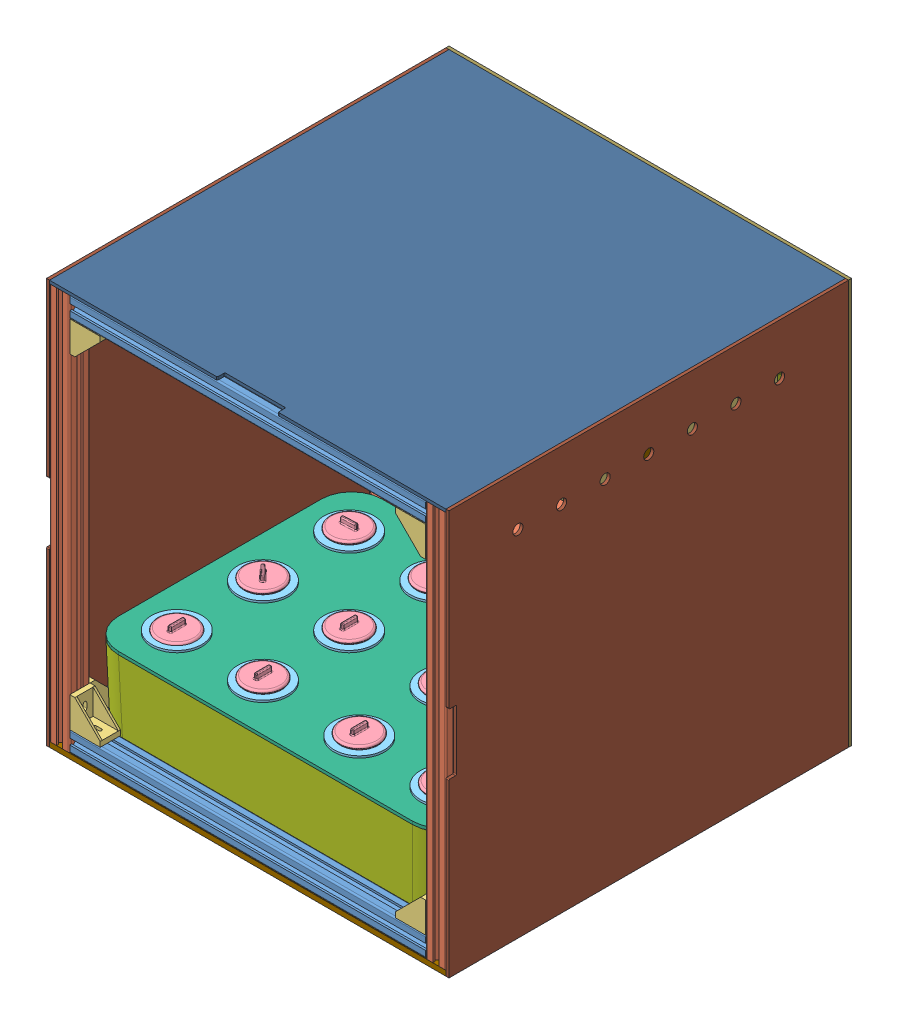
SolidWorks assembly skeleton_v2, configuration 預設. Lengths in mm.
Overall size (397 399 397).
120 component instances, 60 part files, 439 mates.
Components (placement in the parent):
- stick_2020_340-1: stick_2020_340 [預設] at (-3.9446 -1.8678 340) size (20 20 351)
- stick_2020_380-1: stick_2020_380 [預設] at (-3.9446 379.1322 701) x (0 0 1) z (0 -1 0) size (20 20 391)
- stick_2020_340-2: stick_2020_340 [預設] at (357.0554 -1.8678 701) x (0 0 1) z (-1 0 0) size (20 20 351)
- stick_2020_340-3: stick_2020_340 [預設] at (-3.9446 369.1322 340) size (20 20 351)
- stick_2020_340-4: stick_2020_340 [預設] at (357.0554 369.1322 701) x (0 0 1) z (-1 0 0) size (20 20 351)
- stick_2020_340-5: stick_2020_340 [預設] at (357.0554 369.1322 330) x (0 0 1) z (-1 0 0) size (20 20 351)
- stick_2020_340-6: stick_2020_340 [預設] at (367.0554 -1.8678 691) x (-1 0 0) z (0 0 -1) size (20 20 351)
- stick_2020_340-7: stick_2020_340 [預設] at (367.0554 369.1322 691) x (-1 0 0) z (0 0 -1) size (20 20 351)
- stick_2020_340-8: stick_2020_340 [預設] at (6.0554 -1.8678 330) x (0 -1 0) z (1 0 0) size (20 20 351)
- stick_2020_380-2: stick_2020_380 [預設] at (-3.9446 379.1322 330) x (0 0 1) z (0 -1 0) size (20 20 391)
- stick_2020_380-3: stick_2020_380 [預設] at (367.0554 379.1322 701) x (0 0 1) z (0 -1 0) size (20 20 391)
- stick_2020_380-4: stick_2020_380 [預設] at (367.0554 379.1322 330) x (0 0 1) z (0 -1 0) size (20 20 391)
- 零件2^skeleton_v2-1: 零件2^skeleton_v2 [預設] at origin (virtual)
- FixedcomponentWithtriright-2: FixedcomponentWithtriright [預設] at (287.8736 343.8981 342.3593) x (0 -1 0) z (0 0 1) size (81.36 80.18 24)
- small lid-1: small lid [預設] at (48.5554 83.1322 562.9859) x (-0.71803 0 0.696012) z (-0.696012 0 -0.71803) size (38 19 38)
- small lid-2: small lid [預設] at (48.5554 81.1322 647.9859) size (38 19 38)
- small lid-4: small lid [預設] at (228.5554 83.1322 477.9859) x (0.923727 0 0.383052) z (-0.383052 0 0.923727) size (38 19 38)
- small lid-5: small lid [預設] at (228.5554 83.1322 647.9859) size (38 19 38)
- small lid-6: small lid [預設] at (48.5554 83.1322 477.9859) x (0.040502 0 0.999179) z (-0.999179 0 0.040502) size (38 19 38)
- small lid-7: small lid [預設] at (133.5554 83.1322 562.9859) size (38 19 38)
- small lid-8: small lid [預設] at (228.5554 83.1322 562.9859) x (0.921959 0 0.387288) z (-0.387288 0 0.921959) size (38 19 38)
- small lid-9: small lid [預設] at (313.5554 83.1322 647.9859) size (38 19 38)
- small lid-10: small lid [預設] at (133.5554 83.1322 477.9859) x (0.981055 0 -0.193727) z (0.193727 0 0.981055) size (38 19 38)
- small lid-11: small lid [預設] at (133.5554 83.1322 647.9859) size (38 19 38)
- ring-2: ring [預設] at (48.5554 81.1322 562.9859) x (-0.846172 0 0.53291) z (-0.53291 0 -0.846172) size (49.5 5.25 49.5)
- ring-3: ring [預設] at (48.5554 81.1322 647.9859) x (0.619769 0 0.784784) z (-0.784784 0 0.619769) size (49.5 5.25 49.5)
- ring-6: ring [預設] at (133.5554 81.1322 477.9859) x (0.017137 0 0.999853) z (-0.999853 0 0.017137) size (49.5 5.25 49.5)
- ring-9: ring [預設] at (133.5554 81.1322 562.9859) size (49.5 5.25 49.5)
- ring-10: ring [預設] at (133.5554 81.1322 647.9859) x (0.510723 0 0.859745) z (-0.859745 0 0.510723) size (49.5 5.25 49.5)
- ring-11: ring [預設] at (313.5554 81.1322 477.9859) size (49.5 5.25 49.5)
- ring-12: ring [預設] at (313.5554 81.1322 562.9859) size (49.5 5.25 49.5)
- ring-13: ring [預設] at (228.5554 81.1322 647.9859) size (49.5 5.25 49.5)
- ring-14: ring [預設] at (228.5554 81.1322 562.9859) size (49.5 5.25 49.5)
- ring-15: ring [預設] at (228.5554 81.1322 477.9859) size (49.5 5.25 49.5)
- ring-16: ring [預設] at (313.5554 81.1322 647.9859) size (49.5 5.25 49.5)
- ring-17: ring [預設] at (48.5554 81.1322 477.9859) x (0.560642 0 0.828058) z (-0.828058 0 0.560642) size (49.5 5.25 49.5)
- lid_v2-1: lid_v2 [預設] at (181.0554 78.1322 562.9859) size (350 3 260)
- water_tank_v3-1: water_tank_v3 [預設] at (181.0554 -11.8678 562.9859) size (350 90 260)
- small fixed lid with EC sensor and temperture-3: small fixed lid with EC sensor and temperture [預設] at (313.5554 85.1322 562.9859) x (0.682945 0 -0.73047) z (0.73047 0 0.682945) size (38.59 9 40.38)
- plate_bottom-1: plate_bottom [預設] at (181.5554 -16.8678 514) size (391 5 394)
- plate_back-1: plate_back [預設] at (181.5554 183.6322 317) size (391 391 3) (hidden)
- plate_top-1: plate_top [預設] at (181.5554 379.1322 514) size (391 3 394)
- plate_side-1: plate_side [預設] at (-16.9446 182.6322 514) size (3 399 394)
- plate_side-2: plate_side [預設] at (377.0554 182.6322 514) size (3 399 394)
- plate_door-2: plate_door [預設] at (181.5554 182.6322 314) size (397 399 3)
- FixedcomponentWithtri-2: FixedcomponentWithtri [預設] at (61.2372 343.8805 342.3593) x (0 -1 0) z (0 0 1) size (81.36 80.18 24)
- Fixedcomponent_middle-31: Fixedcomponent_middle [預設] at (66.2372 343.8805 342.3593) x (0 -1 0) z (0 0 1) size (51.61 140 24)
- Fixedcomponent_left-43: Fixedcomponent_left [預設] at (21.3071 97.7683 342.3593) size (51.61 200 24)
- Fixedcomponent_right-43: Fixedcomponent_right [預設] at (341.8036 297.7859 342.3593) x (-1 0 0) z (0 0 1) size (51.61 200 24)
- Assem1-1: Assem1 [Default] at (204.6254 174.6149 298.8159) x (-1 0 0) z (0 0 1) size (30 30 12.25)
  - raspberry pi test-1: raspberry pi test [Default] at (8.841 -5.913 4.088) size (30 30 11.7)
  - last-1: last [Default] at (25.9241 1.0773 75.1482) x (-1 0 0) z (0 0 -1) size (30 30 4.5)
  - Raspberry Pi  Camera-1: Raspberry Pi  Camera [Default] at (13.1383 15.2285 23.1841) x (-1 0 0) z (0 0 1) size (25 24 6)
- 1219 ControlBox version-1: 1219 ControlBox version [預設] at (317.0991 120.1322 388.759) x (-1 0 0) z (0 -1 0) size (88 82 106.01)
  - 1219 third floor-1: 1219 third floor [預設] at (8.7787 40.759 112.8702) x (1 0 0) z (0 0 -1) size (81.6 37.75 81.6)
  - 1219 second floor-1: 1219 second floor [預設] at (8.7787 -23.241 112.8702) x (1 0 0) z (0 0 -1) size (81.6 8 81.6)
  - 1219 ground-1: 1219 ground [預設] at (0.3623 -33.241 92.6228) size (88 72 88)
  - 1219 roof-1: 1219 roof [預設] at (-3.5854 48.759 93.9882) x (1 0 0) z (0 0 -1) size (88 10 88)
  - STM32 fixed board-1: STM32 fixed board [預設] at (7.9161 -18.241 103.3439) x (-1 0 0) z (0 1 0) size (70.08 30 1.8)
  - EC and PH support-3: EC and PH support [預設] at (25.441 -20.241 60.8804) x (-0.837169 0 -0.546944) z (-0.546944 0 0.837169) size (4 3 2)
  - The small Fixed board on the converter-1: The small Fixed board on the converter [預設] at (21.8123 17.059 74.3493) x (0 0 -1) z (-1 0 0) size (46.7 1.6 58.25)
  - M3_20mm_pillar-1: M3_20mm_pillar [預設] at (12.0438 39.859 57) x (-0.990685 0 -0.13617) z (-0.13617 0 0.990685) size (6 22.8 6)
  - M3_20mm_pillar-2: M3_20mm_pillar [預設] at (28.2938 39.859 87.2) x (0.837169 0 0.546944) z (0.546944 0 -0.837169) size (6 22.8 6)
  - 12VLEDconnector-1: 12VLEDconnector [預設] at (41.8438 -2.8554 76.5711) x (0 1 0) z (-1 0 0) size (12 37 6.2)
  - O2-1: O2 [預設] at (-12.6825 28.759 117.8445) x (-1 0 0) z (0 1 0) size (37 27 19)
  - JQC3F-1: JQC3F [預設] at (-14.4789 35.759 60.4222) x (1 0 0.000244) z (0 -1 0) size (33.51 25.73 16.5)
  - LM2596 DC to DC Buck Converter 3 A-1: LM2596 DC to DC Buck Converter 3 A [預設] at (20.1688 38.759 72.1) x (0 0 -1) z (-1 0 0) size (43.2 15.15 21.25)
    - LM2596 DC to DC Buck Converter 3 A.STEP-1: LM2596 DC to DC Buck Converter 3 A.STEP [預設] at origin size (43.2 15.15 21.25)
      - lm2596board.STEP-1: lm2596board.STEP [預設] at origin size (43.2 1.71 21.25)
      - smd100uF.STEP-1: smd100uF.STEP [預設] at (-17.25 2.55 0) x (0 0 -1) z (1 0 0) size (11.2 9.76 8.2)
      - smd220uF.STEP-1: smd220uF.STEP [預設] at (17.25 2.55 0) x (0 0 -1) z (1 0 0) size (11.2 9.76 8.2)
      - TrimmerW203.STEP-1: TrimmerW203.STEP [預設] at (4.6271 6.95 -9.1276) size (9.5 15.15 4.81)
      - smdS537diode.STEP-1: smdS537diode.STEP [預設] at (-9.35 1.75 8.875) x (-1 0 0) z (0 0 -1) size (6.5 2.06 2.5)
      - smdceramiccapacitor.STEP-1: smdceramiccapacitor.STEP [預設] at (-15 1.7 5.7969) x (0 0 1) z (-1 0 0) size (2.52 0.61 1.3)
      - smdceramiccapacitor.STEP-2: smdceramiccapacitor.STEP [預設] at (-1.3196 1.7 -5.2916) x (0 0 1) z (-1 0 0) size (2.52 0.61 1.3)
      - smdResistor331.STEP-1: smdResistor331.STEP [預設] at (-1.2696 1.7 -8.4665) x (0 0 1) z (-1 0 0) size (2.53 0.63 1.31)
      - smdResistor102.STEP-1: smdResistor102.STEP [預設] at (10.7771 1.7 -8.4665) x (0 0 -1) z (1 0 0) size (2.53 0.63 1.31)
      - smdLED.STEP-1: smdLED.STEP [預設] at (13.0521 1.75 -8.4701) x (0 0 -1) z (1 0 0) size (3.23 0.86 1.26)
      - smbInductor470.STEP-1: smbInductor470.STEP [預設] at (3.1271 2.1 3.175) size (12.5 7.41 12.5)
      - LM2596S.STEP-1: LM2596S.STEP [預設] at (-8.0627 1.8 -4.5407) size (9.8 4.61 14.95)
  - SCD30_CO2-1: SCD30_CO2 [預設] at (27.7597 38.759 111.9487) x (1 0 0) z (0 -1 0) size (35 23 13)
  - EC and PH support-1: EC and PH support [預設] at (-14.5186 -20.241 69.2115) x (-0.837169 0 -0.546944) z (-0.546944 0 0.837169) size (4 3 2)
  - EC and PH support-2: EC and PH support [預設] at (26.7761 -17.241 71.7105) x (-0.837169 0 -0.546944) z (-0.546944 0 0.837169) size (4 3 2)
  - Gravity Dissolved Oxygen Sensor v1.0.step-1: Gravity Dissolved Oxygen Sensor v1.0.step [預設] at (20.5726 -17.241 68.5206) x (-0.001647 0 0.999999) z (0 1 0) size (63.5 32 13.2)
  - PH-4502C.STEP-1: PH-4502C.STEP [預設] at (-10.49 -8.3658 14.8331) x (0.023795 0 -0.999717) z (0.999717 0 0.023795) size (69.21 20.03 32.26)
    - Board_ph.STEP-1: Board_ph.STEP [預設] at (-41.1248 -11.8752 -79.7631) size (42 1.6 32)
    - BNC_90.STEP-1: BNC_90.STEP [預設] at (-42.729 11.0976 0.372) x (-0.000016 0 -1) z (0 -1 0) size (13 30 18)
    - Trimpot multivoltas_Valor predeterminado.STEP-1: Trimpot multivoltas_Valor predeterminado.STEP [預設] at (-58.9938 -5.1252 9.5069) x (-1 0 0) z (0 0 -1) size (9.8 15.4 5)
    - Trimpot multivoltas_Valor predeterminado.STEP-2: Trimpot multivoltas_Valor predeterminado.STEP [預設] at (-44.5735 -5.1252 13.9129) size (9.8 15.4 5)
    - pin_header_6.STEP-1: pin_header_6.STEP [預設] at (-71.799 -14.5822 4.6019) size (10.45 8.64 15.24)
    - S08.stp.STEP-1: S08.stp.STEP [預設] at (-63.5983 -10.4552 -1.493) x (1 0 0) z (0 1 0) size (4.9 6 1.55)
    - S08.stp.STEP-2: S08.stp.STEP [預設] at (-47.5601 -10.4552 -15.9552) x (-0.008727 0 0.999962) z (0 1 0) size (4.9 6 1.55)
    - S08.stp.STEP-3: S08.stp.STEP [預設] at (-45.4779 -10.4552 -0.8959) x (-0.999848 0 -0.017452) z (0 1 0) size (4.9 6 1.55)
    - ptc.STEP-1: ptc.STEP [預設] at (-58.5127 -8.5499 -13.3623) x (0 -1 0) z (0 0 -1) size (11.73 9.76 5.87)
  - STM32 Nucleo-32-1: STM32 Nucleo-32 [預設] at (17.5119 -16.441 114.2714) x (1 0 0) z (0 1 0) size (50.29 18.54 16)
  - JQC3F -2-1: JQC3F -2 [預設] at (-15.4815 35.759 86.544) x (1 0 0.000244) z (0 -1 0) size (34 26.5 16.5)
  - DC socket-1: DC socket [Default] at (45.0438 -1.491 76.492) x (0 1 0) z (1 0 0) size (9.4 15 14.3)
  - YELLOW JST XH 3 PIN CONNECTOR - P 2.54mm - ANGLED.stp-1: YELLOW JST XH 3 PIN CONNECTOR - P 2.54mm - ANGLED.stp [預設] at (19.2438 12.609 53.8153) x (0 -1 0) z (1 0 0) size (8.73 7.46 10.34)
  - YELLOW JST XH 4 PIN CONNECTOR - P 2.54mm - ANGLED.stp-1: YELLOW JST XH 4 PIN CONNECTOR - P 2.54mm - ANGLED.stp [預設] at (-12.5062 12.609 53.8153) x (0 -1 0) z (1 0 0) size (8.73 7.46 12.88)
- controlbox_left-1: controlbox_left [預設] at (116.0554 -11.8678 386.5) x (-1 0 0) z (0 0 -1) size (220 83 93)
- controlbox_lid-1: controlbox_lid [預設] at (116.1055 71.1322 386.7449) x (0.999995 0 0.003061) z (-0.003061 0 0.999995) size (220 10 93)
- Aluminium extrusion connector-1: Aluminium extrusion connector [預設] at (-13.9446 359.1322 370) x (0 -1 0) z (-1 0 0) size (30 30 20)
- Aluminium extrusion connector-15: Aluminium extrusion connector [預設] at (6.0554 329.1322 320) x (1 0 0) z (0 0 -1) size (30 30 20)
- Aluminium extrusion connector-13: Aluminium extrusion connector [預設] at (-13.9446 38.1322 340) x (0 0 1) z (-1 0 0) size (30 30 20)
- Aluminium extrusion connector-17: Aluminium extrusion connector [預設] at (6.0554 38.1322 340) size (30 30 20)
- Aluminium extrusion connector-12: Aluminium extrusion connector [預設] at (357.0554 38.1322 691) x (-1 0 0) z (0 0 -1) size (30 30 20)
- Aluminium extrusion connector-14: Aluminium extrusion connector [預設] at (377.0554 38.1322 691) x (0 0 -1) z (1 0 0) size (30 30 20)
- Aluminium extrusion connector-5: Aluminium extrusion connector [預設] at (357.0554 359.1322 370) x (0 -1 0) z (-1 0 0) size (30 30 20)
- Aluminium extrusion connector-10: Aluminium extrusion connector [預設] at (327.0554 359.1322 320) x (0 -1 0) z (0 0 -1) size (30 30 20)
- Aluminium extrusion connector-7: Aluminium extrusion connector [預設] at (377.0554 8.1322 370) x (0 1 0) z (1 0 0) size (30 30 20)
- Aluminium extrusion connector-16: Aluminium extrusion connector [預設] at (357.0554 38.1322 320) x (-1 0 0) z (0 0 -1) size (30 30 20)
- Aluminium extrusion connector-2: Aluminium extrusion connector [預設] at (357.0554 329.1322 711) x (-1 0 0) z (0 0 1) size (30 30 20)
- Aluminium extrusion connector-3: Aluminium extrusion connector [預設] at (327.0554 379.1322 691) x (0 0 -1) z (0 1 0) size (30 30 20)
- Aluminium extrusion connector-4: Aluminium extrusion connector [預設] at (377.0554 359.1322 661) x (0 -1 0) z (1 0 0) size (30 30 20)
- Aluminium extrusion connector-6: Aluminium extrusion connector [預設] at (-13.9446 329.1322 691) x (0 0 -1) z (-1 0 0) size (30 30 20)
- Aluminium extrusion connector-8: Aluminium extrusion connector [預設] at (6.0554 379.1322 661) x (1 0 0) z (0 1 0) size (30 30 20)
- Aluminium extrusion connector-20: Aluminium extrusion connector [預設] at (36.0554 359.1322 711) x (0 -1 0) z (0 0 1) size (30 30 20)
- Aluminium extrusion connector-18: Aluminium extrusion connector [預設] at (6.0554 38.1322 711) size (30 30 20)
- Aluminium extrusion connector-19: Aluminium extrusion connector [預設] at (6.0554 38.1322 691) x (0 0 -1) z (1 0 0) size (30 30 20)
- small fixed lid with PH sensor and water leverl-1: small fixed lid with PH sensor and water leverl [預設] at (313.5554 85.1322 477.9859) x (0.999117 0 -0.04201) z (0.04201 0 0.999117) size (38.59 9 40.38)
Mates (geometry in assembly coordinates):
- 重合/共線/共點1: coincident anti-aligned: plane of stick_2020_340-1 through (-3.9446 -1.8678 691) normal (0 0 1); plane of stick_2020_380-1 through (-13.9446 -11.8678 691) normal (0 0 -1)
- 重合/共線/共點2: coincident aligned: line of stick_2020_340-1 through (-12.4446 -11.8678 691) axis (1 0 0); line of stick_2020_380-1 through (-12.4446 -11.8678 691) axis (1 0 0)
- 重合/共線/共點4: coincident: plane of stick_2020_340-1 through (-13.9446 8.1322 691) normal (-1 0 0); line of stick_2020_380-1 through (-13.9446 -11.8678 709.5) axis (0 0 -1)
- 重合/共線/共點5: coincident anti-aligned: plane of stick_2020_380-1 through (6.0554 -11.8678 691) normal (1 0 0); plane of stick_2020_340-2 through (6.0554 -1.8678 701) normal (-1 0 0)
- 重合/共線/共點6: coincident: plane of stick_2020_380-1 through (-13.9446 -11.8678 711) normal (0 0 1); line of stick_2020_340-2 through (6.0554 -10.3678 711) axis (0 1 0)
- 重合/共線/共點7: coincident: line of stick_2020_380-1 through (6.0554 -11.8678 692.5) axis (0 0 1); plane of stick_2020_340-2 through (6.0554 -11.8678 691) normal (0 -1 0)
- 重合/共線/共點8: coincident anti-aligned: plane of stick_2020_380-1 through (-13.9446 -11.8678 691) normal (0 0 -1); plane of stick_2020_340-3 through (-3.9446 369.1322 691) normal (0 0 1)
- 重合/共線/共點9: coincident: plane of stick_2020_380-1 through (-3.9446 379.1322 701) normal (0 1 0); line of stick_2020_340-3 through (4.5554 379.1322 691) axis (-1 0 0)
- 重合/共線/共點10: coincident aligned: plane of stick_2020_380-1 through (6.0554 -11.8678 691) normal (1 0 0); plane of stick_2020_340-3 through (6.0554 379.1322 691) normal (1 0 0)
- 重合/共線/共點11: coincident aligned: plane of stick_2020_380-1 through (-3.9446 379.1322 701) normal (0 1 0); plane of stick_2020_340-4 through (6.0554 379.1322 691) normal (0 1 0)
- 重合/共線/共點12: coincident aligned: plane of stick_2020_380-1 through (-13.9446 -11.8678 711) normal (0 0 1); plane of stick_2020_340-4 through (6.0554 379.1322 711) normal (0 0 1)
- 重合/共線/共點13: coincident anti-aligned: plane of stick_2020_380-1 through (6.0554 -11.8678 691) normal (1 0 0); plane of stick_2020_340-4 through (6.0554 369.1322 701) normal (-1 0 0)
- 重合/共線/共點17: coincident anti-aligned: plane of stick_2020_340-3 through (-3.9446 369.1322 340) normal (0 0 -1); plane of stick_2020_380-2 through (-13.9446 -11.8678 340) normal (0 0 1)
- 重合/共線/共點18: coincident aligned: plane of stick_2020_340-3 through (-13.9446 379.1322 691) normal (0 1 0); plane of stick_2020_380-2 through (-3.9446 379.1322 330) normal (0 1 0)
- 重合/共線/共點19: coincident aligned: plane of stick_2020_340-3 through (6.0554 379.1322 691) normal (1 0 0); plane of stick_2020_380-2 through (6.0554 -11.8678 320) normal (1 0 0)
- 重合/共線/共點20: coincident aligned: plane of stick_2020_340-5 through (6.0554 379.1322 320) normal (0 1 0); plane of stick_2020_380-2 through (-3.9446 379.1322 330) normal (0 1 0)
- 重合/共線/共點21: coincident anti-aligned: plane of stick_2020_340-5 through (6.0554 369.1322 330) normal (-1 0 0); plane of stick_2020_380-2 through (6.0554 -11.8678 320) normal (1 0 0)
- 重合/共線/共點22: coincident aligned: plane of stick_2020_340-5 through (6.0554 379.1322 320) normal (0 0 -1); plane of stick_2020_380-2 through (-13.9446 -11.8678 320) normal (0 0 -1)
- 重合/共線/共點23: coincident aligned: plane of stick_2020_340-4 through (6.0554 379.1322 691) normal (0 1 0); plane of stick_2020_380-3 through (367.0554 379.1322 701) normal (0 1 0)
- 重合/共線/共點24: coincident anti-aligned: plane of stick_2020_340-4 through (357.0554 369.1322 701) normal (1 0 0); plane of stick_2020_380-3 through (357.0554 -11.8678 691) normal (-1 0 0)
- 重合/共線/共點26: coincident aligned: plane of stick_2020_340-4 through (6.0554 379.1322 691) normal (0 0 -1); plane of stick_2020_380-3 through (357.0554 -11.8678 691) normal (0 0 -1)
- 重合/共線/共點27: coincident anti-aligned: plane of stick_2020_340-6 through (367.0554 -1.8678 691) normal (0 0 1); plane of stick_2020_380-3 through (357.0554 -11.8678 691) normal (0 0 -1)
- 重合/共線/共點28: coincident aligned: plane of stick_2020_340-6 through (377.0554 8.1322 340) normal (1 0 0); plane of stick_2020_380-3 through (377.0554 -11.8678 691) normal (1 0 0)
- 重合/共線/共點29: coincident aligned: plane of stick_2020_340-6 through (377.0554 -11.8678 340) normal (0 -1 0); plane of stick_2020_380-3 through (367.0554 -11.8678 701) normal (0 -1 0)
- 重合/共線/共點30: coincident anti-aligned: plane of stick_2020_340-7 through (367.0554 369.1322 691) normal (0 0 1); plane of stick_2020_380-3 through (357.0554 -11.8678 691) normal (0 0 -1)
- 重合/共線/共點31: coincident aligned: plane of stick_2020_340-7 through (377.0554 379.1322 340) normal (1 0 0); plane of stick_2020_380-3 through (377.0554 -11.8678 691) normal (1 0 0)
- 重合/共線/共點32: coincident aligned: plane of stick_2020_340-7 through (377.0554 379.1322 340) normal (0 1 0); plane of stick_2020_380-3 through (367.0554 379.1322 701) normal (0 1 0)
- 重合/共線/共點33: coincident aligned: plane of stick_2020_340-5 through (6.0554 379.1322 320) normal (0 1 0); plane of stick_2020_380-4 through (367.0554 379.1322 330) normal (0 1 0)
- 重合/共線/共點35: coincident anti-aligned: plane of stick_2020_340-7 through (367.0554 369.1322 340) normal (0 0 -1); plane of stick_2020_380-4 through (357.0554 -11.8678 340) normal (0 0 1)
- 重合/共線/共點36: coincident aligned: plane of stick_2020_340-7 through (377.0554 379.1322 340) normal (1 0 0); plane of stick_2020_380-4 through (377.0554 -11.8678 320) normal (1 0 0)
- 重合/共線/共點38: coincident anti-aligned: plane of stick_2020_340-8 through (6.0554 -1.8678 330) normal (-1 0 0); plane of stick_2020_380-2 through (6.0554 -11.8678 320) normal (1 0 0)
- 重合/共線/共點39: coincident aligned: plane of stick_2020_340-8 through (357.0554 8.1322 320) normal (0 0 -1); plane of stick_2020_380-2 through (-13.9446 -11.8678 320) normal (0 0 -1)
- 重合/共線/共點40: coincident aligned: plane of stick_2020_340-6 through (377.0554 -11.8678 340) normal (0 -1 0); plane of stick_2020_340-8 through (357.0554 -11.8678 320) normal (0 -1 0)
- 重合/共線/共點43: coincident anti-aligned: plane of stick_2020_380-1 through (6.0554 -11.8678 691) normal (1 0 0); plane of tri-1 through (6.0554 28.1322 709.5) normal (-1 0 0)
- 重合/共線/共點44: coincident anti-aligned: plane of stick_2020_340-2 through (6.0554 8.1322 691) normal (0 1 0); plane of tri-1 through (6.0554 8.1322 709.5) normal (0 -1 0)
- 重合/共線/共點45: coincident: line of stick_2020_380-1 through (6.0554 379.1322 709.5) axis (0 -1 0); plane of tri-1 through (6.0554 8.1322 709.5) normal (0 0 1)
- 重合/共線/共點46: coincident anti-aligned: plane of stick_2020_380-1 through (-13.9446 -11.8678 691) normal (0 0 -1); plane of tri-9 through (4.5554 28.1322 691) normal (0 0 1)
- 重合/共線/共點47: coincident anti-aligned: plane of stick_2020_340-1 through (-13.9446 8.1322 691) normal (0 1 0); plane of tri-9 through (4.5554 8.1322 691) normal (0 -1 0)
- 重合/共線/共點48: coincident: line of stick_2020_380-1 through (-12.4446 -11.8678 691) axis (0 1 0); plane of tri-9 through (-12.4446 8.1322 691) normal (-1 0 0)
- 重合/共線/共點49: coincident anti-aligned: plane of stick_2020_340-1 through (6.0554 8.1322 691) normal (1 0 0); plane of tri-10 through (6.0554 6.6322 670) normal (-1 0 0)
- 重合/共線/共點50: coincident anti-aligned: plane of stick_2020_340-2 through (6.0554 8.1322 691) normal (0 0 -1); plane of tri-10 through (6.0554 6.6322 690) normal (0 0 1)
- 重合/共線/共點51: coincident: line of stick_2020_340-1 through (6.0554 -10.3678 691) axis (0 0 -1); plane of tri-10 through (6.0554 -10.3678 690) normal (0 -1 0)
- 重合/共線/共點52: coincident anti-aligned: plane of stick_2020_340-2 through (6.0554 8.1322 691) normal (0 1 0); plane of tri-3 through (357.0554 8.1322 692.5) normal (0 -1 0)
- 重合/共線/共點54: coincident anti-aligned: plane of stick_2020_380-3 through (357.0554 -11.8678 691) normal (-1 0 0); plane of tri-3 through (357.0554 28.1322 692.5) normal (1 0 0)
- 重合/共線/共點55: coincident: line of stick_2020_380-3 through (357.0554 -11.8678 709.5) axis (0 1 0); plane of tri-3 through (357.0554 8.1322 709.5) normal (0 0 1)
- 重合/共線/共點56: coincident anti-aligned: plane of stick_2020_380-3 through (357.0554 -11.8678 691) normal (0 0 -1); plane of tri-4 through (375.5554 28.1322 691) normal (0 0 1)
- 重合/共線/共點57: coincident anti-aligned: plane of stick_2020_340-6 through (377.0554 8.1322 340) normal (0 1 0); plane of tri-4 through (375.5554 8.1322 691) normal (0 -1 0)
- 重合/共線/共點58: coincident: line of stick_2020_380-3 through (375.5554 379.1322 691) axis (0 -1 0); plane of tri-4 through (375.5554 8.1322 691) normal (1 0 0)
- 重合/共線/共點59: coincident anti-aligned: plane of stick_2020_340-2 through (6.0554 8.1322 691) normal (0 0 -1); plane of tri-5 through (356.0554 -10.3678 690) normal (0 0 1)
- 重合/共線/共點61: coincident anti-aligned: plane of stick_2020_340-6 through (357.0554 8.1322 340) normal (-1 0 0); plane of tri-5 through (356.0554 -10.3678 670) normal (1 0 0)
- 重合/共線/共點62: coincident: line of stick_2020_340-2 through (357.0554 -10.3678 691) axis (-1 0 0); plane of tri-5 through (356.0554 -10.3678 690) normal (0 -1 0)
- 重合/共線/共點63: coincident anti-aligned: plane of stick_2020_380-2 through (-13.9446 -11.8678 340) normal (0 0 1); plane of tri-8 through (-12.4446 28.1322 340) normal (0 0 -1)
- 重合/共線/共點64: coincident: line of stick_2020_380-2 through (-12.4446 379.1322 340) axis (0 -1 0); plane of tri-8 through (-12.4446 8.1322 340) normal (-1 0 0)
- 重合/共線/共點65: coincident anti-aligned: plane of stick_2020_340-1 through (-13.9446 8.1322 691) normal (0 1 0); plane of tri-8 through (-12.4446 8.1322 340) normal (0 -1 0)
- 重合/共線/共點66: coincident anti-aligned: plane of stick_2020_380-2 through (6.0554 -11.8678 320) normal (1 0 0); plane of tri-2 through (6.0554 28.1322 338.5) normal (-1 0 0)
- 重合/共線/共點67: coincident anti-aligned: plane of stick_2020_340-8 through (357.0554 8.1322 320) normal (0 1 0); plane of tri-2 through (6.0554 8.1322 338.5) normal (0 -1 0)
- 重合/共線/共點68: coincident: line of stick_2020_340-8 through (357.0554 8.1322 321.5) axis (-1 0 0); plane of tri-2 through (6.0554 8.1322 321.5) normal (0 0 -1)
- 重合/共線/共點69: coincident anti-aligned: plane of stick_2020_340-1 through (6.0554 8.1322 691) normal (1 0 0); plane of tri-7 through (6.0554 -10.3678 360) normal (-1 0 0)
- 重合/共線/共點70: coincident anti-aligned: plane of stick_2020_340-8 through (357.0554 8.1322 340) normal (0 0 1); plane of tri-7 through (6.0554 -10.3678 340) normal (0 0 -1)
- 重合/共線/共點71: coincident: line of stick_2020_340-1 through (6.0554 -10.3678 691) axis (0 0 -1); plane of tri-7 through (6.0554 -10.3678 340) normal (0 -1 0)
- 重合/共線/共點72: coincident anti-aligned: plane of stick_2020_380-4 through (357.0554 -11.8678 320) normal (-1 0 0); plane of tri-6 through (357.0554 28.1322 321.5) normal (1 0 0)
- 重合/共線/共點73: coincident anti-aligned: plane of stick_2020_380-4 through (357.0554 -11.8678 320) normal (-1 0 0); plane of tri-6 through (357.0554 28.1322 321.5) normal (1 0 0)
- 重合/共線/共點77: coincident: line of stick_2020_380-4 through (357.0554 379.1322 321.5) axis (0 -1 0); plane of tri-6 through (357.0554 8.1322 321.5) normal (0 0 -1)
- 重合/共線/共點78: coincident anti-aligned: plane of stick_2020_340-8 through (357.0554 8.1322 320) normal (0 1 0); plane of tri-6 through (357.0554 8.1322 321.5) normal (0 -1 0)
- 重合/共線/共點79: coincident anti-aligned: plane of stick_2020_380-4 through (357.0554 -11.8678 340) normal (0 0 1); plane of tri-11 through (358.5554 28.1322 340) normal (0 0 -1)
- 重合/共線/共點80: coincident: line of stick_2020_380-4 through (358.5554 379.1322 340) axis (0 -1 0); plane of tri-11 through (358.5554 8.1322 340) normal (-1 0 0)
- 重合/共線/共點81: coincident anti-aligned: plane of stick_2020_340-6 through (377.0554 8.1322 340) normal (0 1 0); plane of tri-11 through (358.5554 8.1322 340) normal (0 -1 0)
- 重合/共線/共點83: coincident anti-aligned: plane of stick_2020_340-6 through (357.0554 8.1322 340) normal (-1 0 0); plane of tri-12 through (356.0554 6.6322 360) normal (1 0 0)
- 重合/共線/共點84: coincident anti-aligned: plane of stick_2020_340-8 through (357.0554 8.1322 340) normal (0 0 1); plane of tri-12 through (356.0554 6.6322 340) normal (0 0 -1)
- 重合/共線/共點85: coincident: line of stick_2020_340-6 through (357.0554 6.6322 691) axis (0 0 -1); plane of tri-12 through (356.0554 6.6322 340) normal (0 1 0)
- 重合/共線/共點86: coincident anti-aligned: plane of stick_2020_380-4 through (357.0554 -11.8678 320) normal (-1 0 0); plane of tri-23 through (357.0554 339.1322 338.5) normal (1 0 0)
- 重合/共線/共點87: coincident anti-aligned: plane of stick_2020_340-5 through (6.0554 359.1322 320) normal (0 -1 0); plane of tri-23 through (357.0554 359.1322 338.5) normal (0 1 0)
- 重合/共線/共點88: coincident: line of stick_2020_340-5 through (357.0554 359.1322 338.5) axis (-1 0 0); plane of tri-23 through (357.0554 359.1322 338.5) normal (0 0 1)
- 重合/共線/共點89: coincident anti-aligned: plane of stick_2020_340-7 through (357.0554 379.1322 340) normal (-1 0 0); plane of tri-17 through (357.0554 377.6322 360) normal (1 0 0)
- 重合/共線/共點90: coincident anti-aligned: plane of stick_2020_340-5 through (6.0554 379.1322 340) normal (0 0 1); plane of tri-17 through (357.0554 377.6322 340) normal (0 0 -1)
- 重合/共線/共點91: coincident: line of stick_2020_340-5 through (357.0554 377.6322 340) axis (-1 0 0); plane of tri-17 through (357.0554 377.6322 340) normal (0 1 0)
- 重合/共線/共點92: coincident anti-aligned: plane of stick_2020_380-4 through (357.0554 -11.8678 340) normal (0 0 1); plane of tri-22 through (375.5554 339.1322 340) normal (0 0 -1)
- 重合/共線/共點93: coincident anti-aligned: plane of stick_2020_340-7 through (377.0554 359.1322 340) normal (0 -1 0); plane of tri-22 through (375.5554 359.1322 340) normal (0 1 0)
- 重合/共線/共點94: coincident: line of stick_2020_340-7 through (375.5554 359.1322 340) axis (0 0 1); plane of tri-22 through (375.5554 359.1322 340) normal (1 0 0)
- 重合/共線/共點100: coincident anti-aligned: plane of stick_2020_340-5 through (6.0554 379.1322 340) normal (0 0 1); plane of tri-24 through (6.0554 360.6322 340) normal (0 0 -1)
- 重合/共線/共點101: coincident anti-aligned: plane of stick_2020_340-3 through (6.0554 379.1322 691) normal (1 0 0); plane of tri-24 through (6.0554 360.6322 360) normal (-1 0 0)
- 重合/共線/共點102: coincident: line of stick_2020_340-5 through (357.0554 377.6322 340) axis (-1 0 0); plane of tri-24 through (6.0554 377.6322 340) normal (0 1 0)
- 重合/共線/共點103: coincident anti-aligned: plane of stick_2020_340-5 through (6.0554 359.1322 320) normal (0 -1 0); plane of tri-20 through (6.0554 359.1322 321.5) normal (0 1 0)
- 重合/共線/共點104: coincident anti-aligned: plane of stick_2020_380-2 through (6.0554 -11.8678 320) normal (1 0 0); plane of tri-20 through (6.0554 339.1322 321.5) normal (-1 0 0)
- 重合/共線/共點105: coincident: line of stick_2020_340-5 through (6.0554 359.1322 321.5) axis (1 0 0); plane of tri-20 through (6.0554 359.1322 321.5) normal (0 0 -1)
- 重合/共線/共點106: coincident anti-aligned: plane of stick_2020_340-3 through (-13.9446 359.1322 691) normal (0 -1 0); plane of tri-19 through (4.5554 359.1322 340) normal (0 1 0)
- 重合/共線/共點107: coincident anti-aligned: plane of stick_2020_380-2 through (-13.9446 -11.8678 340) normal (0 0 1); plane of tri-19 through (4.5554 339.1322 340) normal (0 0 -1)
- 重合/共線/共點108: coincident: line of stick_2020_340-3 through (-12.4446 359.1322 691) axis (0 0 -1); plane of tri-19 through (-12.4446 359.1322 340) normal (-1 0 0)
- 重合/共線/共點109: coincident anti-aligned: plane of stick_2020_380-1 through (-13.9446 -11.8678 691) normal (0 0 -1); plane of tri-13 through (4.5554 359.1322 691) normal (0 0 1)
- 重合/共線/共點110: coincident anti-aligned: plane of stick_2020_340-3 through (-13.9446 359.1322 691) normal (0 -1 0); plane of tri-13 through (4.5554 359.1322 671) normal (0 1 0)
- 重合/共線/共點111: coincident: line of stick_2020_380-1 through (-12.4446 -11.8678 691) axis (0 1 0); plane of tri-13 through (-12.4446 359.1322 691) normal (-1 0 0)
- 重合/共線/共點112: coincident anti-aligned: plane of stick_2020_340-4 through (6.0554 379.1322 691) normal (0 0 -1); plane of tri-18 through (6.0554 377.6322 691) normal (0 0 1)
- 重合/共線/共點113: coincident anti-aligned: plane of stick_2020_340-3 through (6.0554 379.1322 691) normal (1 0 0); plane of tri-18 through (6.0554 377.6322 671) normal (-1 0 0)
- 重合/共線/共點114: coincident: line of stick_2020_340-3 through (6.0554 377.6322 340) axis (0 0 1); plane of tri-18 through (6.0554 377.6322 691) normal (0 1 0)
- 重合/共線/共點115: coincident anti-aligned: plane of stick_2020_380-1 through (6.0554 -11.8678 691) normal (1 0 0); plane of tri-15 through (6.0554 339.1322 692.5) normal (-1 0 0)
- 重合/共線/共點116: coincident anti-aligned: plane of stick_2020_340-4 through (6.0554 359.1322 691) normal (0 -1 0); plane of tri-15 through (6.0554 359.1322 692.5) normal (0 1 0)
- 重合/共線/共點117: coincident: line of stick_2020_380-1 through (6.0554 379.1322 709.5) axis (0 -1 0); plane of tri-15 through (6.0554 359.1322 709.5) normal (0 0 1)
- 重合/共線/共點118: coincident anti-aligned: plane of stick_2020_340-7 through (357.0554 379.1322 340) normal (-1 0 0); plane of tri-14 through (357.0554 377.6322 691) normal (1 0 0)
- 重合/共線/共點119: coincident anti-aligned: plane of stick_2020_340-4 through (6.0554 379.1322 691) normal (0 0 -1); plane of tri-14 through (337.0554 377.6322 691) normal (0 0 1)
- 重合/共線/共點120: coincident: line of stick_2020_340-4 through (6.0554 377.6322 691) axis (1 0 0); plane of tri-14 through (357.0554 377.6322 691) normal (0 1 0)
- 重合/共線/共點121: coincident anti-aligned: plane of stick_2020_380-3 through (357.0554 -11.8678 691) normal (0 0 -1); plane of tri-21 through (375.5554 359.1322 691) normal (0 0 1)
- 重合/共線/共點123: coincident anti-aligned: plane of stick_2020_340-7 through (377.0554 359.1322 340) normal (0 -1 0); plane of tri-21 through (375.5554 359.1322 671) normal (0 1 0)
- 重合/共線/共點124: coincident: line of stick_2020_340-7 through (358.5554 359.1322 691) axis (0 0 -1); plane of tri-21 through (358.5554 359.1322 691) normal (-1 0 0)
- 重合/共線/共點125: coincident anti-aligned: plane of stick_2020_380-3 through (357.0554 -11.8678 691) normal (-1 0 0); plane of tri-16 through (357.0554 359.1322 692.5) normal (1 0 0)
- 重合/共線/共點126: coincident anti-aligned: plane of stick_2020_340-4 through (6.0554 359.1322 691) normal (0 -1 0); plane of tri-16 through (337.0554 359.1322 692.5) normal (0 1 0)
- 重合/共線/共點127: coincident: line of stick_2020_380-3 through (357.0554 -11.8678 709.5) axis (0 1 0); plane of tri-16 through (357.0554 359.1322 709.5) normal (0 0 1)
- 重合/共線/共點132: coincident anti-aligned: plane of stick_2020_340-1 through (6.0554 8.1322 691) normal (1 0 0); plane of water_tank_copy-1 through (6.0554 78.1322 684.3736) normal (-1 0 0)
- 重合/共線/共點133: coincident aligned: plane of stick_2020_340-8 through (357.0554 -11.8678 320) normal (0 -1 0); plane of water_tank_copy-1 through (181.0554 -11.8678 554.3736) normal (0 -1 0)
- 相切1: tangent anti-aligned: cylinder of tri-10; cylinder of water_tank_copy-1 through (36.0554 78.1322 654.3736) axis (0 -1 0) radius 30
- 重合/共線/共點135: coincident aligned: plane of water_tank_copy-1 through (356.0554 78.1322 684.3736) normal (1 0 0); plane of lid_v2-1 through (356.0554 81.1322 692.9859) normal (1 0 0)
- 重合/共線/共點136: coincident aligned: plane of water_tank_copy-1 through (6.0554 78.1322 684.3736) normal (0 0 1); plane of lid_v2-1 through (6.0554 81.1322 692.9859) normal (0 0 1)
- 重合/共線/共點140: coincident anti-aligned: plane of stick_2020_340-6 through (377.0554 8.1322 340) normal (0 1 0); plane of angle-1 through (326.0554 8.1322 454.3736) normal (0 -1 0)
- 重合/共線/共點141: coincident aligned: plane of stick_2020_340-6 through (377.0554 8.1322 340) normal (1 0 0); plane of angle-1 through (376.0554 28.1322 422.8736) normal (1 0 0)
- 同軸心1: concentric aligned: cylinder of water_tank_copy-1 through (326.0554 78.1322 454.3736) axis (0 -1 0) radius 30; cylinder of angle-1 through (326.0554 28.1322 454.3736) axis (0 -1 0) radius 30
- 重合/共線/共點142: coincident anti-aligned: plane of lid_v2-1 through (181.0554 81.1322 562.9859) normal (0 1 0); plane of ring-1 through (48.5554 81.1322 477.9859) normal (0 -1 0)
- 重合/共線/共點143: coincident anti-aligned: plane of lid_v2-1 through (181.0554 81.1322 562.9859) normal (0 1 0); plane of ring-2 through (48.5554 81.1322 562.9859) normal (0 -1 0)
- 重合/共線/共點144: coincident anti-aligned: plane of lid_v2-1 through (181.0554 81.1322 562.9859) normal (0 1 0); plane of ring-3 through (48.5554 81.1322 647.9859) normal (0 -1 0)
- 重合/共線/共點146: coincident anti-aligned: plane of lid_v2-1 through (181.0554 81.1322 562.9859) normal (0 1 0); plane of ring-6 through (133.5554 81.1322 477.9859) normal (0 -1 0)
- 重合/共線/共點147: coincident anti-aligned: plane of lid_v2-1 through (181.0554 81.1322 562.9859) normal (0 1 0); plane of ring-9 through (133.5554 81.1322 562.9859) normal (0 -1 0)
- 重合/共線/共點149: coincident anti-aligned: plane of lid_v2-1 through (181.0554 81.1322 562.9859) normal (0 1 0); plane of ring-10 through (133.5554 81.1322 647.9859) normal (0 -1 0)
- 重合/共線/共點150: coincident anti-aligned: plane of stick_2020_340-1 through (-13.9446 8.1322 691) normal (0 1 0); plane of angle-2 through (36.0554 8.1322 391.3736) normal (0 -1 0)
- 重合/共線/共點151: coincident aligned: plane of stick_2020_340-1 through (-13.9446 8.1322 691) normal (-1 0 0); plane of angle-2 through (-13.9446 28.1322 422.8736) normal (-1 0 0)
- 同軸心10: concentric aligned: cylinder of water_tank_copy-1 through (36.0554 78.1322 454.3736) axis (0 -1 0) radius 30; cylinder of angle-2 through (36.0554 28.1322 454.3736) axis (0 -1 0) radius 30
- 重合/共線/共點158: coincident aligned: plane of water_tank_copy-1 through (181.0554 -11.8678 554.3736) normal (0 -1 0); plane of controlbox_left-7 through (106.0554 -11.8678 383.4986) normal (0 -1 0)
- 重合/共線/共點159: coincident aligned: plane of water_tank_copy-1 through (6.0554 78.1322 684.3736) normal (-1 0 0); plane of controlbox_left-7 through (6.0554 78.1322 345.6236) normal (-1 0 0)
- 同軸心12: concentric aligned: cylinder of angle-2 through (36.0554 28.1322 391.3736) axis (0 -1 0) radius 30; cylinder of controlbox_left-7 through (36.0554 78.1322 391.3736) axis (0 -1 0) radius 30
- 重合/共線/共點167: coincident aligned: plane of controlbox_right-3 through (106.0554 -11.8678 386.5) normal (0 -1 0); plane of controlbox_middle-1 through (181.0554 -11.8678 386.5) normal (0 -1 0)
- 重合/共線/共點168: coincident anti-aligned: plane of controlbox_right-3 through (106.0554 78.1322 433) normal (-1 0 0); plane of controlbox_middle-1 through (256.0554 78.1322 433) normal (1 0 0)
- 重合/共線/共點170: coincident anti-aligned: plane of stick_2020_340-8 through (357.0554 8.1322 320) normal (0 1 0); plane of tri_back-1 through (168.9592 8.1322 339.9936) normal (0 -1 0)
- 重合/共線/共點174: coincident anti-aligned: plane of stick_2020_340-1 through (-13.9446 8.1322 691) normal (0 1 0); plane of angle_v2-2 through (-13.9446 8.1322 430.5551) normal (0 -1 0)
- 重合/共線/共點175: coincident aligned: plane of stick_2020_340-1 through (-13.9446 8.1322 691) normal (-1 0 0); plane of angle_v2-2 through (-13.9446 28.1322 397.5551) normal (-1 0 0)
- 重合/共線/共點178: coincident: line of stick_2020_340-2 through (6.0554 6.6322 691) axis (1 0 0); plane of water_tank_v3-1 through (6.0554 78.1322 692.9859) normal (0 -0.027765 0.999614)
- 重合/共線/共點179: coincident aligned: plane of stick_2020_340-2 through (6.0554 -11.8678 691) normal (0 -1 0); plane of water_tank_v3-1 through (181.0554 -11.8678 562.9859) normal (0 -1 0)
- 重合/共線/共點185: coincident anti-aligned: plane of stick_2020_340-6 through (377.0554 8.1322 340) normal (0 1 0); plane of angle_v2-1 through (376.0554 8.1322 433.4082) normal (0 -1 0)
- 重合/共線/共點190: coincident: plane of stick_2020_340-1 through (6.0554 8.1322 691) normal (1 0 0); line of water_tank_v3-1 through (6.0554 78.1322 462.9744) axis (0 0 1)
- 重合/共線/共點195: coincident aligned: plane of stick_2020_340-6 through (377.0554 8.1322 340) normal (1 0 0); plane of angle_v2-1 through (376.0554 28.1322 463.4082) normal (1 0 0)
- 重合/共線/共點197: coincident aligned: line of lid_v2-1 through (36.0554 78.1322 692.9859) axis (1 0 0); line of water_tank_v3-1 through (36.0438 78.1322 692.9859) axis (1 0 0)
- 重合/共線/共點198: coincident aligned: line of lid_v2-1 through (6.0554 78.1322 462.9859) axis (0 0 1); line of water_tank_v3-1 through (6.0554 78.1322 462.9744) axis (0 0 1)
- 重合/共線/共點200: coincident anti-aligned: plane of stick_2020_340-8 through (357.0554 8.1322 340) normal (0 0 1); plane of controlbox_middle-1 through (106.0554 78.1322 340) normal (0 0 -1)
- 重合/共線/共點201: coincident aligned: plane of stick_2020_340-8 through (357.0554 -11.8678 320) normal (0 -1 0); plane of controlbox_middle-1 through (181.0554 -11.8678 386.5) normal (0 -1 0)
- 重合/共線/共點203: coincident aligned: plane of stick_2020_340-8 through (357.0554 -11.8678 320) normal (0 -1 0); plane of controlbox_left-1 through (116.0554 -11.8678 386.5) normal (0 -1 0)
- 重合/共線/共點204: coincident anti-aligned: plane of stick_2020_340-1 through (-13.9446 8.1322 691) normal (0 1 0); plane of angle_v3-1 through (-13.9446 8.1322 431.9462) normal (0 -1 0)
- 重合/共線/共點205: coincident aligned: plane of stick_2020_340-1 through (-13.9446 8.1322 691) normal (-1 0 0); plane of angle_v3-1 through (-13.9446 78.1322 401.9098) normal (-1 0 0)
- 重合/共線/共點206: coincident anti-aligned: plane of stick_2020_340-1 through (-13.9446 8.1322 691) normal (0 1 0); plane of angle_v3-2 through (-13.9446 8.1322 431.5412) normal (0 -1 0)
- 重合/共線/共點207: coincident aligned: plane of stick_2020_340-1 through (-13.9446 8.1322 691) normal (-1 0 0); plane of angle_v3-2 through (-13.9446 78.1322 401.4412) normal (-1 0 0)
- 重合/共線/共點208: coincident anti-aligned: plane of stick_2020_340-1 through (-13.9446 8.1322 691) normal (0 1 0); plane of angle_v4-1 through (-13.9446 8.1322 432.0174) normal (0 -1 0)
- 重合/共線/共點209: coincident aligned: plane of stick_2020_340-1 through (-13.9446 8.1322 691) normal (-1 0 0); plane of angle_v4-1 through (-13.9446 78.1322 402.0174) normal (-1 0 0)
- 重合/共線/共點210: coincident aligned: plane of stick_2020_340-6 through (377.0554 8.1322 340) normal (1 0 0); plane of angle-right-1 through (377.0554 78.1322 462.1124) normal (1 0 0)
- 重合/共線/共點211: coincident anti-aligned: plane of stick_2020_340-6 through (377.0554 8.1322 340) normal (0 1 0); plane of angle-right-1 through (377.0554 8.1322 432.1124) normal (0 -1 0)
- 重合/共線/共點212: coincident anti-aligned: plane of stick_2020_340-1 through (-13.9446 8.1322 691) normal (0 1 0); plane of angle-left-1 through (-13.9446 8.1322 432.1954) normal (0 -1 0)
- 重合/共線/共點213: coincident aligned: plane of stick_2020_340-1 through (-13.9446 8.1322 691) normal (-1 0 0); plane of angle-left-1 through (-13.9446 78.1322 402.1954) normal (-1 0 0)
- 重合/共線/共點214: coincident aligned: plane of controlbox_right-3 through (106.0554 78.1322 340) normal (0 0 -1); plane of controlbox_middle-1 through (106.0554 78.1322 340) normal (0 0 -1)
- 同軸心14: concentric aligned: cylinder of lid_v2-1 through (48.5554 78.1312 477.9859) axis (0 1 0) radius 22; cylinder of ring-1 through (48.5554 77.8822 477.9859) axis (0 1 0) radius 21.75
- 同軸心15: concentric aligned: cylinder of lid_v2-1 through (133.5554 78.1312 477.9859) axis (0 1 0) radius 22; cylinder of ring-6 through (133.5554 77.8822 477.9859) axis (0 1 0) radius 21.75
- 重合/共線/共點215: coincident anti-aligned: plane of stick_2020_340-6 through (377.0554 -11.8678 340) normal (0 -1 0); plane of plate_bottom-1 through (181.5554 -11.8678 514) normal (0 1 0)
- 重合/共線/共點217: coincident aligned: plane of stick_2020_340-6 through (377.0554 8.1322 340) normal (1 0 0); plane of plate_bottom-1 through (377.0554 -11.8678 317) normal (1 0 0)
- 同軸心16: concentric aligned: cylinder of lid_v2-1 through (48.5554 78.1312 562.9859) axis (0 1 0) radius 22; cylinder of ring-2 through (48.5554 77.8822 562.9859) axis (0 1 0) radius 21.75
- 同軸心17: concentric aligned: cylinder of lid_v2-1 through (48.5554 78.1312 647.9859) axis (0 1 0) radius 22; cylinder of ring-3 through (48.5554 77.8822 647.9859) axis (0 1 0) radius 21.75
- 同軸心18: concentric aligned: cylinder of lid_v2-1 through (133.5554 78.1312 562.9859) axis (0 1 0) radius 22; cylinder of ring-9 through (133.5554 77.8822 562.9859) axis (0 1 0) radius 21.75
- 同軸心19: concentric aligned: cylinder of lid_v2-1 through (133.5554 78.1312 647.9859) axis (0 1 0) radius 22; cylinder of ring-10 through (133.5554 77.8822 647.9859) axis (0 1 0) radius 21.75
- 重合/共線/共點225: coincident anti-aligned: plane of stick_2020_340-5 through (6.0554 379.1322 320) normal (0 0 -1); plane of plate_back-1 through (181.5554 183.6322 320) normal (0 0 1)
- 重合/共線/共點226: coincident aligned: plane of stick_2020_340-5 through (6.0554 379.1322 320) normal (0 1 0); plane of plate_back-1 through (-13.9446 379.1322 320) normal (0 1 0)
- 重合/共線/共點228: coincident anti-aligned: plane of stick_2020_340-4 through (6.0554 379.1322 691) normal (0 1 0); plane of plate_top-1 through (181.5554 379.1322 514) normal (0 -1 0)
- 重合/共線/共點230: coincident aligned: plane of plate_back-1 through (181.5554 183.6322 317) normal (0 0 -1); plane of plate_top-1 through (-13.9446 382.1322 317) normal (0 0 -1)
- 重合/共線/共點236: coincident aligned: plane of plate_bottom-1 through (-13.9446 -11.8678 317) normal (0 0 -1); plane of plate_back-1 through (181.5554 183.6322 317) normal (0 0 -1)
- 重合/共線/共點237: coincident anti-aligned: plane of controlbox_left-1 through (106.0554 63.1322 340) normal (1 0 0); plane of controlbox_middle-1 through (106.0554 78.1322 433) normal (-1 0 0)
- 重合/共線/共點241: coincident anti-aligned: plane of stick_2020_380-2 through (-13.9446 -11.8678 320) normal (-1 0 0); plane of plate_side-1 through (-13.9446 182.6322 514) normal (1 0 0)
- 重合/共線/共點242: coincident aligned: plane of plate_top-1 through (181.5554 382.1322 514) normal (0 1 0); plane of plate_side-1 through (-13.9446 382.1322 711) normal (0 1 0)
- 重合/共線/共點243: coincident aligned: plane of plate_back-1 through (181.5554 183.6322 317) normal (0 0 -1); plane of plate_side-1 through (-13.9446 382.1322 317) normal (0 0 -1)
- 重合/共線/共點244: coincident anti-aligned: plane of stick_2020_340-7 through (377.0554 379.1322 340) normal (1 0 0); plane of plate_side-2 through (377.0554 182.6322 514) normal (-1 0 0)
- 重合/共線/共點245: coincident aligned: plane of plate_top-1 through (181.5554 382.1322 514) normal (0 1 0); plane of plate_side-2 through (380.0554 382.1322 711) normal (0 1 0)
- 重合/共線/共點247: coincident aligned: plane of plate_back-1 through (181.5554 183.6322 317) normal (0 0 -1); plane of plate_side-2 through (380.0554 382.1322 317) normal (0 0 -1)
- 重合/共線/共點249: coincident anti-aligned: plane of plate_back-1 through (377.0554 379.1322 320) normal (1 0 0); plane of plate_side-2 through (377.0554 182.6322 514) normal (-1 0 0)
- 重合/共線/共點250: coincident aligned: plane of plate_side-1 through (-16.9446 182.6322 514) normal (-1 0 0); plane of plate_door-2 through (-16.9446 382.1322 317) normal (-1 0 0)
- 重合/共線/共點251: coincident aligned: plane of plate_bottom-1 through (181.5554 -16.8678 514) normal (0 -1 0); plane of plate_door-2 through (-16.9446 -16.8678 317) normal (0 -1 0)
- 重合/共線/共點254: coincident anti-aligned: plane of stick_2020_380-3 through (357.0554 -11.8678 691) normal (-1 0 0); plane of magnetic-1 through (357.0554 182.139 700.6422) normal (1 0 0)
- 平行4: parallel aligned: plane of stick_2020_380-3 through (357.0554 -11.8678 711) normal (0 0 1); plane of magnetic-1 through (347.0554 176.139 708.6422) normal (0 0 1)
- 重合/共線/共點255: coincident anti-aligned: plane of plate_side-1 through (-13.9446 182.6322 514) normal (1 0 0); plane of Fixedcomponent-1 through (-13.9446 15.0627 340) normal (-1 0 0)
- 重合/共線/共點256: coincident anti-aligned: plane of plate_back-1 through (181.5554 183.6322 320) normal (0 0 1); plane of Fixedcomponent-1 through (33.6687 15.0627 320) normal (0 0 -1)
- 重合/共線/共點257: coincident anti-aligned: plane of plate_side-1 through (-13.9446 182.6322 514) normal (1 0 0); plane of FixedcomponentWithtri-2 through (-13.9446 328.921 344) normal (-1 0 0)
- 重合/共線/共點258: coincident anti-aligned: plane of plate_top-1 through (181.5554 379.1322 514) normal (0 -1 0); plane of FixedcomponentWithtri-2 through (66.2372 379.1322 340) normal (0 1 0)
- 重合/共線/共點259: coincident anti-aligned: plane of stick_2020_340-5 through (6.0554 379.1322 340) normal (0 0 1); plane of FixedcomponentWithtri-2 through (66.2372 371.3822 340) normal (0 0 -1)
- 重合/共線/共點260: coincident anti-aligned: plane of FixedcomponentWithtri-2 through (10.0054 297.7683 320) normal (0 -1 0); plane of Fixedcomponent_middle-2 through (21.3071 297.7859 342.3593) normal (0 1 0)
- 重合/共線/共點261: coincident aligned: plane of FixedcomponentWithtri-2 through (-13.9446 328.921 344) normal (-1 0 0); plane of Fixedcomponent_middle-2 through (-13.9446 297.7859 340) normal (-1 0 0)
- 重合/共線/共點262: coincident: line of FixedcomponentWithtri-2 through (-13.9446 297.7683 340) axis (1 0 0); plane of Fixedcomponent_middle-2 through (-6.1946 297.7859 340) normal (0 0 -1)
- 重合/共線/共點263: coincident anti-aligned: plane of Fixedcomponent-4 through (341.8036 157.7859 342.3593) normal (0 -1 0); plane of Fixedcomponent_middle-6 through (341.8036 157.7859 342.3593) normal (0 1 0)
- 重合/共線/共點264: coincident aligned: plane of Fixedcomponent-4 through (369.3054 157.7859 340) normal (0 0 -1); plane of Fixedcomponent_middle-6 through (369.3054 17.7859 340) normal (0 0 -1)
- 重合/共線/共點265: coincident aligned: plane of Fixedcomponent-4 through (377.0554 157.7859 340) normal (1 0 0); plane of Fixedcomponent_middle-6 through (377.0554 17.7859 340) normal (1 0 0)
- 重合/共線/共點266: coincident anti-aligned: plane of Fixedcomponent_middle-5 through (341.8036 17.7859 342.3593) normal (0 1 0); plane of Fixedcomponent_middle-6 through (341.8036 17.7859 342.3593) normal (0 -1 0)
- 重合/共線/共點267: coincident aligned: plane of Fixedcomponent-4 through (377.0554 157.7859 340) normal (1 0 0); plane of Fixedcomponent_middle-5 through (377.0554 -122.2141 340) normal (1 0 0)
- 重合/共線/共點268: coincident aligned: plane of Fixedcomponent_middle-5 through (377.0554 -122.2141 344) normal (0 0 1); plane of Fixedcomponent_middle-6 through (377.0554 17.7859 344) normal (0 0 1)
- 重合/共線/共點269: coincident aligned: plane of Fixedcomponent_middle-3 through (377.0554 -262.2141 340) normal (1 0 0); plane of Fixedcomponent_middle-6 through (377.0554 17.7859 340) normal (1 0 0)
- 重合/共線/共點270: coincident anti-aligned: plane of Fixedcomponent_middle-3 through (341.8036 -122.2141 342.3593) normal (0 1 0); plane of Fixedcomponent_middle-5 through (341.8036 -122.2141 342.3593) normal (0 -1 0)
